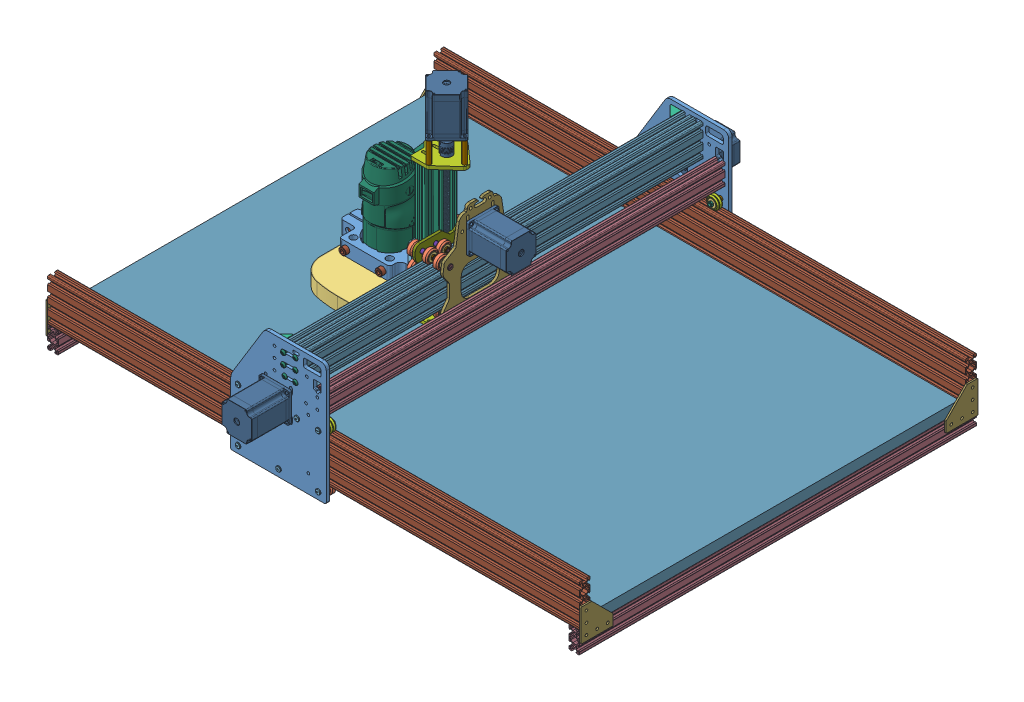
SolidWorks assembly MainFrame, configuration Default. Lengths in mm. (continued)
Components (placement in the parent): (continued)
- V-Slot_Nema23_Z_Build_Plate-1: V-Slot_Nema23_Z_Build_Plate [Default] at (-108.8467 132.9785 -347.7105) x (0 1 0) z (1 0 0) size (382.7 179.74 222.35) (hidden)
  - V-Slot NemaZ Build Plate-1: V-Slot NemaZ Build Plate [Default] at (-20.2121 124.8825 30.9396) size (88 127 2.54)
  - V-Slot Spacer Block-1: V-Slot Spacer Block [Default] at (-73.8059 59.9877 39.4796) x (1 0 0) z (0 0 1) size (86 20 12)
  - V-Slot Spacer Block-2: V-Slot Spacer Block [Default] at (-73.8059 -40.6523 39.4796) size (86 20 12)
  - 8mm Acme Nut Block-1: 8mm Acme Nut Block [Default] at (-83.4859 9.6677 39.4796) x (0 1 0) z (-1 0 0) size (34 12 20.51)
  - SolidWheelWithEccentric2-1: SolidWheelWithEccentric2 [Default] at (-136.732 -45.0423 82.73) x (-0.923728 -0.383049 0) z (0 0 -1) size (23.89 23.89 32.23)
    - SolidWheel-1: SolidWheel [Default] at (5.3595 -13.235 6.1636) size (23.89 23.89 11)
      - Delrin Solid V-Wheel-1: Delrin Solid V-Wheel [Default] at (-37.4558 4.6779 16.5868) size (23.89 23.89 10.23)
      - Precision Ball Bearing-1: Precision Ball Bearing [Default] at (-37.4558 4.6779 19.5868) x (0 0 -1) z (1 0 0) size (5 16 16)
      - Precision Ball Bearing-2: Precision Ball Bearing [Default] at (-37.4558 4.6779 13.5868) x (0 0 1) z (-1 0 0) size (5 16 16)
    - Steel Eccentric Spacer-1: Steel Eccentric Spacer [Default] at (-32.1017 -9.3471 37.2504) x (0 0 -1) z (0.00681 0.999977 0) size (7.27 9.09 7.9)
    - Low Profile Socket Head Screw-1: Low Profile Socket Head Screw [Default] at (-32.0963 -8.5571 45.0004) x (0 0 -1) z (1 0 0) size (32.23 9.5 9.5)
    - hex nut jam_am-1: hex nut jam_am [B18.2.4.5M - Hex jam nut,  M5 x 0.8 --D-N] at (-32.0963 -8.5571 17.2504) size (8 9.24 2.7)
    - 3mm Aluminum Spacer-1: 3mm Aluminum Spacer [Default] at (-32.0963 -8.5571 31.2504) x (0 0 -1) z (1 0 0) size (3 8 8)
  - SolidWheelWithEccentric2-2: SolidWheelWithEccentric2 [Default] at (-76.732 -45.0423 82.73) x (-0.923728 -0.383049 0) z (0 0 -1) size (23.89 23.89 32.23)
    - SolidWheel-1: SolidWheel [Default] at (5.3595 -13.235 6.1636) size (23.89 23.89 11)
      - Delrin Solid V-Wheel-1: Delrin Solid V-Wheel [Default] at (-37.4558 4.6779 16.5868) size (23.89 23.89 10.23)
      - Precision Ball Bearing-1: Precision Ball Bearing [Default] at (-37.4558 4.6779 19.5868) x (0 0 -1) z (1 0 0) size (5 16 16)
      - Precision Ball Bearing-2: Precision Ball Bearing [Default] at (-37.4558 4.6779 13.5868) x (0 0 1) z (-1 0 0) size (5 16 16)
    - Steel Eccentric Spacer-1: Steel Eccentric Spacer [Default] at (-32.1017 -9.3471 37.2504) x (0 0 -1) z (0.00681 0.999977 0) size (7.27 9.09 7.9)
    - Low Profile Socket Head Screw-1: Low Profile Socket Head Screw [Default] at (-32.0963 -8.5571 45.0004) x (0 0 -1) z (1 0 0) size (32.23 9.5 9.5)
    - hex nut jam_am-1: hex nut jam_am [B18.2.4.5M - Hex jam nut,  M5 x 0.8 --D-N] at (-32.0963 -8.5571 17.2504) size (8 9.24 2.7)
    - 3mm Aluminum Spacer-1: 3mm Aluminum Spacer [Default] at (-32.0963 -8.5571 31.2504) x (0 0 -1) z (1 0 0) size (3 8 8)
  - SolidWheelWithSpacer-1: SolidWheelWithSpacer [Default] at (-83.1141 65.4802 73.4636) x (0.923728 0.383049 0) z (0 0 -1) size (23.89 23.89 32.23)
    - SolidWheel-1: SolidWheel [Default] at (16.2383 -7.5303 -3.4528) size (23.89 23.89 11)
      - Delrin Solid V-Wheel-1: Delrin Solid V-Wheel [Default] at (-37.4558 4.6779 16.5868) size (23.89 23.89 10.23)
      - Precision Ball Bearing-1: Precision Ball Bearing [Default] at (-37.4558 4.6779 19.5868) x (0 0 -1) z (1 0 0) size (5 16 16)
      - Precision Ball Bearing-2: Precision Ball Bearing [Default] at (-37.4558 4.6779 13.5868) x (0 0 1) z (-1 0 0) size (5 16 16)
    - Low Profile Socket Head Screw-1: Low Profile Socket Head Screw [Default] at (-21.2174 -2.8524 35.734) x (0 0 -1) z (-0.923728 -0.383049 0) size (32.23 9.5 9.5)
    - .25 Inch Nylon Spacer-1: .25 Inch Nylon Spacer [Default] at (-21.2174 -2.8524 27.984) x (0 0 -1) z (1 0 0) size (6.35 7.94 7.94)
    - hex nut jam_am-1: hex nut jam_am [B18.2.4.5M - Hex jam nut,  M5 x 0.8 --D-N] at (-21.2174 -2.8524 7.634) size (8 9.24 2.7)
    - 3mm Aluminum Spacer-1: 3mm Aluminum Spacer [Default] at (-21.2174 -2.8524 21.634) x (0 0 -1) z (1 0 0) size (3 8 8)
  - SolidWheelWithSpacer-2: SolidWheelWithSpacer [Default] at (-64.4976 54.4952 73.4636) x (-0.923728 -0.383049 0) z (0 0 -1) size (23.89 23.89 32.23)
    - SolidWheel-1: SolidWheel [Default] at (16.2383 -7.5303 -3.4528) size (23.89 23.89 11)
      - Delrin Solid V-Wheel-1: Delrin Solid V-Wheel [Default] at (-37.4558 4.6779 16.5868) size (23.89 23.89 10.23)
      - Precision Ball Bearing-1: Precision Ball Bearing [Default] at (-37.4558 4.6779 19.5868) x (0 0 -1) z (1 0 0) size (5 16 16)
      - Precision Ball Bearing-2: Precision Ball Bearing [Default] at (-37.4558 4.6779 13.5868) x (0 0 1) z (-1 0 0) size (5 16 16)
    - Low Profile Socket Head Screw-1: Low Profile Socket Head Screw [Default] at (-21.2174 -2.8524 35.734) x (0 0 -1) z (-0.923728 -0.383049 0) size (32.23 9.5 9.5)
    - .25 Inch Nylon Spacer-1: .25 Inch Nylon Spacer [Default] at (-21.2174 -2.8524 27.984) x (0 0 -1) z (1 0 0) size (6.35 7.94 7.94)
    - hex nut jam_am-1: hex nut jam_am [B18.2.4.5M - Hex jam nut,  M5 x 0.8 --D-N] at (-21.2174 -2.8524 7.634) size (8 9.24 2.7)
    - 3mm Aluminum Spacer-1: 3mm Aluminum Spacer [Default] at (-21.2174 -2.8524 21.634) x (0 0 -1) z (1 0 0) size (3 8 8)
  - SolidWheelWithSpacer-3: SolidWheelWithSpacer [Default] at (-53.5632 53.0198 73.4636) x (0.980486 -0.196591 0) z (0 0 -1) size (23.89 23.89 32.23)
    - SolidWheel-1: SolidWheel [Default] at (16.2383 -7.5303 -3.4528) size (23.89 23.89 11)
      - Delrin Solid V-Wheel-1: Delrin Solid V-Wheel [Default] at (-37.4558 4.6779 16.5868) size (23.89 23.89 10.23)
      - Precision Ball Bearing-1: Precision Ball Bearing [Default] at (-37.4558 4.6779 19.5868) x (0 0 -1) z (1 0 0) size (5 16 16)
      - Precision Ball Bearing-2: Precision Ball Bearing [Default] at (-37.4558 4.6779 13.5868) x (0 0 1) z (-1 0 0) size (5 16 16)
    - Low Profile Socket Head Screw-1: Low Profile Socket Head Screw [Default] at (-21.2174 -2.8524 35.734) x (0 0 -1) z (-0.923728 -0.383049 0) size (32.23 9.5 9.5)
    - .25 Inch Nylon Spacer-1: .25 Inch Nylon Spacer [Default] at (-21.2174 -2.8524 27.984) x (0 0 -1) z (1 0 0) size (6.35 7.94 7.94)
    - hex nut jam_am-1: hex nut jam_am [B18.2.4.5M - Hex jam nut,  M5 x 0.8 --D-N] at (-21.2174 -2.8524 7.634) size (8 9.24 2.7)
    - 3mm Aluminum Spacer-1: 3mm Aluminum Spacer [Default] at (-21.2174 -2.8524 21.634) x (0 0 -1) z (1 0 0) size (3 8 8)
  - SolidWheelWithEccentric2-3: SolidWheelWithEccentric2 [Default] at (-106.732 -45.0423 82.73) x (-0.923728 -0.383049 0) z (0 0 -1) size (23.89 23.89 32.23)
    - SolidWheel-1: SolidWheel [Default] at (5.3595 -13.235 6.1636) size (23.89 23.89 11)
      - Delrin Solid V-Wheel-1: Delrin Solid V-Wheel [Default] at (-37.4558 4.6779 16.5868) size (23.89 23.89 10.23)
      - Precision Ball Bearing-1: Precision Ball Bearing [Default] at (-37.4558 4.6779 19.5868) x (0 0 -1) z (1 0 0) size (5 16 16)
      - Precision Ball Bearing-2: Precision Ball Bearing [Default] at (-37.4558 4.6779 13.5868) x (0 0 1) z (-1 0 0) size (5 16 16)
    - Steel Eccentric Spacer-1: Steel Eccentric Spacer [Default] at (-32.1017 -9.3471 37.2504) x (0 0 -1) z (0.00681 0.999977 0) size (7.27 9.09 7.9)
    - Low Profile Socket Head Screw-1: Low Profile Socket Head Screw [Default] at (-32.0963 -8.5571 45.0004) x (0 0 -1) z (1 0 0) size (32.23 9.5 9.5)
    - hex nut jam_am-1: hex nut jam_am [B18.2.4.5M - Hex jam nut,  M5 x 0.8 --D-N] at (-32.0963 -8.5571 17.2504) size (8 9.24 2.7)
    - 3mm Aluminum Spacer-1: 3mm Aluminum Spacer [Default] at (-32.0963 -8.5571 31.2504) x (0 0 -1) z (1 0 0) size (3 8 8)
  - 8mm TR8_8 Leadscrew-1: 8mm TR8_8 Leadscrew [1000mm - Default] at (-183.0043 9.6677 39.2196) x (0 0 1) z (-1 0 0) size (8.21 8.21 254)
  - V-Slot 20mm x 80mm x 300mm-1: V-Slot 20mm x 80mm x 300mm [Default] at (-184.3543 39.8452 60.1696) x (0 0 1) z (-1 0 0) size (20 80.02 250)
  - V-Slot Threaded Rod Plate-Nema23-1: V-Slot Threaded Rod Plate-Nema23 [Default] at (65.6457 -0.3323 60.1696) x (0 1 0) z (1 0 0) size (80 77.5 6.35)
  - V-Slot Threaded Rod Plate-Nema23-2: V-Slot Threaded Rod Plate-Nema23 [Default] at (-184.3543 19.6677 60.1696) x (0 -1 0) z (-1 0 0) size (80 77.5 6.35) (hidden)
  - stepper motor NEMA 23 57x76-1: stepper motor NEMA 23 57x76 [По умолчанию] at (186.9957 9.6677 39.2196) x (0 0.707107 -0.707107) z (0 0.707107 0.707107) size (56.67 96.5 56.58)
  - 40mm Aluminum Spacer-1: 40mm Aluminum Spacer [Default] at (111.9957 -23.9906 39.2196) x (-1 0 0) z (0 0.924225 0.381849) size (40 8 8)
  - 40mm Aluminum Spacer-2: 40mm Aluminum Spacer [Default] at (111.9957 9.6677 5.5613) x (-1 0 0) z (0 0.924225 0.381849) size (40 8 8)
  - 40mm Aluminum Spacer-3: 40mm Aluminum Spacer [Default] at (111.9957 43.326 39.2196) x (-1 0 0) z (0 0.924225 0.381849) size (40 8 8)
  - 40mm Aluminum Spacer-4: 40mm Aluminum Spacer [Default] at (111.9957 9.6677 72.8779) x (-1 0 0) z (0 0.924225 0.381849) size (40 8 8)
  - socket head cap screw_am-1: socket head cap screw_am [B18.3.1M - 5 x 0.8 x 25 Hex SHCS -- 25NHX] at (76.9957 -20.1748 60.1696) x (-1 0 0) z (0 -0.384278 0.923217) size (30 8.5 8.5)
  - socket head cap screw_am-2: socket head cap screw_am [B18.3.1M - 5 x 0.8 x 25 Hex SHCS -- 25NHX] at (76.9957 -0.1748 60.1696) x (-1 0 0) z (0 -0.700437 0.713714) size (30 8.5 8.5)
  - socket head cap screw_am-3: socket head cap screw_am [B18.3.1M - 5 x 0.8 x 25 Hex SHCS -- 25NHX] at (76.9957 19.8452 60.1696) x (-1 0 0) z (0 0.86302 0.50517) size (30 8.5 8.5)
  - socket head cap screw_am-4: socket head cap screw_am [B18.3.1M - 5 x 0.8 x 25 Hex SHCS -- 25NHX] at (76.9957 39.8452 60.1696) x (-1 0 0) z (0 0 1) size (30 8.5 8.5)
  - socket head cap screw_am-6: socket head cap screw_am [B18.3.1M - 5 x 0.8 x 25 Hex SHCS -- 25NHX] at (-195.7043 -20.1748 60.1696) x (1 0 0) z (0 0 1) size (30 8.5 8.5)
  - socket head cap screw_am-7: socket head cap screw_am [B18.3.1M - 5 x 0.8 x 25 Hex SHCS -- 25NHX] at (-195.7043 -0.1748 60.1696) x (1 0 0) z (0 0 1) size (30 8.5 8.5)
  - socket head cap screw_am-8: socket head cap screw_am [B18.3.1M - 5 x 0.8 x 25 Hex SHCS -- 25NHX] at (-195.7043 19.8452 60.1696) x (1 0 0) z (0 0 1) size (30 8.5 8.5)
  - socket head cap screw_am-9: socket head cap screw_am [B18.3.1M - 5 x 0.8 x 25 Hex SHCS -- 25NHX] at (-195.7043 39.8452 60.1696) x (1 0 0) z (0 0 1) size (30 8.5 8.5)
  - socket head cap screw_am-10: socket head cap screw_am [B18.3.1M - 4 x 0.7 x 55 Hex SHCS -- 20NHX] at (120.9957 -23.9906 39.2196) x (-1 0 0) z (0 0.924225 0.381849) size (59 7 7)
  - socket head cap screw_am-11: socket head cap screw_am [B18.3.1M - 4 x 0.7 x 55 Hex SHCS -- 20NHX] at (120.9957 9.6677 5.5613) x (-1 0 0) z (0 0 1) size (59 7 7)
  - socket head cap screw_am-12: socket head cap screw_am [B18.3.1M - 4 x 0.7 x 55 Hex SHCS -- 20NHX] at (120.9957 43.326 39.2196) x (-1 0 0) z (0 0 1) size (59 7 7)
  - socket head cap screw_am-13: socket head cap screw_am [B18.3.1M - 4 x 0.7 x 55 Hex SHCS -- 20NHX] at (120.9957 9.6677 72.8779) x (-1 0 0) z (0 0 1) size (59 7 7)
  - 5mm x 8mm Flexible Coupling-1: 5mm x 8mm Flexible Coupling [Default] at (76.9957 9.6677 39.2196) x (0 0 1) z (-1 0 0) size (20.7 20.83 25.02)
  - BoschRouter-1: BoschRouter [Default] at (-190.8659 -31.4315 -23.846) x (0 0 1) z (0 1 0) size (186 234.6 179.74) (hidden)
    - Main router body-1: Main router body [Default] at (-10.2226 84.5551 41.0992) size (99.4 181.94 153.51)
    - Part2^BoschRouter-1: Part2^BoschRouter [Default] at (-10.2226 69.8231 41.0992) x (-0.837169 0 -0.546944) z (-0.546944 0 0.837169) size (16.99 12.7 21.58) (virtual)
    - 0.25 in ENDMILL-1: 0.25 in ENDMILL [Default] at (-10.3095 59.0843 40.9903) x (-0.983799 0 0.179276) z (0.179276 0 0.983799) size (6.8 68.83 6.97)
    - pan cross head_ai-1: pan cross head_ai [CR-PHMS 0.138-32x0.375x0.375-N] at (-1.965 82.0913 10.6382) x (0 1 0) z (0 0 1) size (11.95 6.86 6.86)
    - pan cross head_ai-2: pan cross head_ai [CR-PHMS 0.138-32x0.375x0.375-N] at (-41.774 82.0913 41.8547) x (0 1 0) z (0 0 1) size (11.95 6.86 6.86)
    - pan cross head_ai-3: pan cross head_ai [CR-PHMS 0.138-32x0.375x0.375-N] at (9.6999 82.0913 65.5768) x (0 1 0) z (0 0 1) size (11.95 6.86 6.86)
    - BoschRouterMount-1: BoschRouterMount [Default] at (-10.2226 84.5551 41.0992) x (-1 0 0) z (0 -1 0) size (140 100 25)
    - socket head cap screw_am-1: socket head cap screw_am [B18.3.1M - 8 x 1.25 x 30 Hex SHCS -- 30NHX] at (-70.2144 97.0551 17.7105) x (0 0 1) z (0.923728 0.383049 0) size (38 13 13)
    - BoschRouter-ShoeRods-1: BoschRouter-ShoeRods [Default] at (-10.2226 109.5551 41.0992) x (1 0 0) z (0 1 0) size (80.73 12.7 110)
    - BoschRouter-ShowPlate-1: BoschRouter-ShowPlate [Default] at (-10.2226 32.6551 41.0992) x (-1 0 0) z (0 -1 0) size (162 139.64 25.4)
    - socket head cap screw_am-2: socket head cap screw_am [B18.3.1M - 8 x 1.25 x 12 Hex SHCS -- 12NHX] at (26.3004 97.0551 98.7105) x (0 0 -1) z (1 0 0) size (20 13 13)
    - socket head cap screw_am-3: socket head cap screw_am [B18.3.1M - 8 x 1.25 x 12 Hex SHCS -- 12NHX] at (-41.7291 97.0551 98.7105) x (0 0 -1) z (1 0 0) size (20 13 13)
    - socket head cap screw_am-4: socket head cap screw_am [B18.3.1M - 8 x 1.25 x 12 Hex SHCS -- 12NHX] at (26.3004 97.0551 -17.2895) x (0 0 1) z (-1 0 0) size (20 13 13)
    - socket head cap screw_am-5: socket head cap screw_am [B18.3.1M - 8 x 1.25 x 12 Hex SHCS -- 12NHX] at (-41.7291 97.0551 -17.2895) x (0 0 1) z (-1 0 0) size (20 13 13)
    - BoschRouter-ShoeVacumPort-1: BoschRouter-ShoeVacumPort [Default] at (-10.2226 32.6551 41.0992) x (1 0 0) z (0 1 0) size (45 45 44.53)
    - RouterMountingPlate-2: RouterMountingPlate [Default] at (-25.2226 46.2551 41.0992) x (1 0 0) z (0 1 0) size (6.35 60 101.6)
    - socket head cap screw_am-6: socket head cap screw_am [B18.3.1M - 5 x 0.8 x 12 Hex SHCS -- 12NHX] at (49.7856 137.8551 61.0992) size (17 8.5 8.5)
    - socket head cap screw_am-7: socket head cap screw_am [B18.3.1M - 5 x 0.8 x 12 Hex SHCS -- 12NHX] at (49.7856 137.8551 41.0992) size (17 8.5 8.5)
    - socket head cap screw_am-8: socket head cap screw_am [B18.3.1M - 5 x 0.8 x 12 Hex SHCS -- 12NHX] at (49.7856 137.8551 21.0992) size (17 8.5 8.5)
    - socket head cap screw_am-9: socket head cap screw_am [B18.3.1M - 5 x 0.8 x 12 Hex SHCS -- 12NHX] at (49.7856 56.2551 21.0992) x (1 0 0) z (0 0 -1) size (17 8.5 8.5)
    - socket head cap screw_am-10: socket head cap screw_am [B18.3.1M - 5 x 0.8 x 12 Hex SHCS -- 12NHX] at (49.7856 56.2551 61.0992) size (17 8.5 8.5)
    - socket head cap screw_am-11: socket head cap screw_am [B18.3.1M - 5 x 0.8 x 12 Hex SHCS -- 12NHX] at (49.7856 56.2551 41.0992) size (17 8.5 8.5)
  - V-Slot_Bottom_Threaded_Rod_Plate-Nema23-1: V-Slot_Bottom_Threaded_Rod_Plate-Nema23 [Default] at (-184.3543 19.6677 60.1696) x (0 -1 0) z (-1 0 0) size (80 45 6.35)
  - R4-ZZ Ball Bearing-1: R4-ZZ Ball Bearing [Default] at (-184.8651 9.6677 39.2196) x (1 0 0) z (0 0 1) size (4.98 10 10)
  - R4-ZZ Ball Bearing-2: R4-ZZ Ball Bearing [Default] at (65.1349 9.6677 39.2196) x (1 0 0) z (0 0.062023 0.998075) size (4.98 10 10)
- 5 Hole 90 Degree Joining Plate-1: 5 Hole 90 Degree Joining Plate [Default] at (-476.3518 -111.2884 -724.722) x (0 0 1) z (-0.999999 -0.001454 0) size (60 60 3)
- 5 Hole 90 Degree Joining Plate-2: 5 Hole 90 Degree Joining Plate [Default] at (-473.3518 -111.284 21.278) x (0 0 -1) z (0.999999 0.001454 0) size (60 60 3)
- 5 Hole 90 Degree Joining Plate-3: 5 Hole 90 Degree Joining Plate [Default] at (526.6471 -109.8153 -724.7365) x (0.000002 -0.001454 0.999999) z (-0.999999 -0.001454 0) size (60 60 3)
- 5 Hole 90 Degree Joining Plate-4: 5 Hole 90 Degree Joining Plate [Default] at (529.6471 -109.8255 21.278) x (0 0 -1) z (0.999999 0.001454 0) size (60 60 3)
- V-Slot 20mm x 40mm x BedCrossBrace-1: V-Slot 20mm x 40mm x BedCrossBrace [Default] at (516.632 -99.4444 21.278) x (0.999999 0.001454 0) z (0 0 1) size (20 40 746)
- V-Slot 20mm x 40mm x BedCrossBrace-4: V-Slot 20mm x 40mm x BedCrossBrace [Default] at (-463.367 -100.8695 21.278) x (0.999999 0.001454 0) z (0 0 1) size (20 40 746)
- HoldDownBoard-1: HoldDownBoard [Default] at (196.6178 -89.9123 21.278) x (0.999999 0.001454 0) z (-0.001454 0.999999 0) size (1000 680.6 19.05)
- BoschRouter-2: BoschRouter [Default] at (-136.4727 -50.9445 -335.8021) x (1 0 0) z (0 -0.000396 1) size (186 234.6 179.74)
  - Main router body-1: Main router body [Default] at (-10.2226 84.5551 41.0992) size (99.4 181.94 153.51)
  - Part2^BoschRouter-1: Part2^BoschRouter [Default] at (-10.2226 69.8231 41.0992) x (-0.837169 0 -0.546944) z (-0.546944 0 0.837169) size (16.99 12.7 21.58) (virtual)
  - 0.25 in ENDMILL-1: 0.25 in ENDMILL [Default] at (-10.3095 59.0843 40.9903) x (-0.983799 0 0.179276) z (0.179276 0 0.983799) size (6.8 68.83 6.97)
  - pan cross head_ai-1: pan cross head_ai [CR-PHMS 0.138-32x0.375x0.375-N] at (-1.965 82.0913 10.6382) x (0 1 0) z (0 0 1) size (11.95 6.86 6.86)
  - pan cross head_ai-2: pan cross head_ai [CR-PHMS 0.138-32x0.375x0.375-N] at (-41.774 82.0913 41.8547) x (0 1 0) z (0 0 1) size (11.95 6.86 6.86)
  - pan cross head_ai-3: pan cross head_ai [CR-PHMS 0.138-32x0.375x0.375-N] at (9.6999 82.0913 65.5768) x (0 1 0) z (0 0 1) size (11.95 6.86 6.86)
  - BoschRouterMount-1: BoschRouterMount [Default] at (-10.2226 84.5551 41.0992) x (-1 0 0) z (0 -1 0) size (140 100 25)
  - socket head cap screw_am-1: socket head cap screw_am [B18.3.1M - 8 x 1.25 x 30 Hex SHCS -- 30NHX] at (-70.2144 97.0551 17.7105) x (0 0 1) z (0.923728 0.383049 0) size (38 13 13)
  - BoschRouter-ShoeRods-1: BoschRouter-ShoeRods [Default] at (-10.2226 109.5551 41.0992) x (1 0 0) z (0 1 0) size (80.73 12.7 110)
  - BoschRouter-ShowPlate-1: BoschRouter-ShowPlate [Default] at (-10.2226 32.6551 41.0992) x (-1 0 0) z (0 -1 0) size (162 139.64 25.4)
  - socket head cap screw_am-2: socket head cap screw_am [B18.3.1M - 8 x 1.25 x 12 Hex SHCS -- 12NHX] at (26.3004 97.0551 98.7105) x (0 0 -1) z (1 0 0) size (20 13 13)
  - socket head cap screw_am-3: socket head cap screw_am [B18.3.1M - 8 x 1.25 x 12 Hex SHCS -- 12NHX] at (-41.7291 97.0551 98.7105) x (0 0 -1) z (1 0 0) size (20 13 13)
  - socket head cap screw_am-4: socket head cap screw_am [B18.3.1M - 8 x 1.25 x 12 Hex SHCS -- 12NHX] at (26.3004 97.0551 -17.2895) x (0 0 1) z (-1 0 0) size (20 13 13)
  - socket head cap screw_am-5: socket head cap screw_am [B18.3.1M - 8 x 1.25 x 12 Hex SHCS -- 12NHX] at (-41.7291 97.0551 -17.2895) x (0 0 1) z (-1 0 0) size (20 13 13)
  - BoschRouter-ShoeVacumPort-1: BoschRouter-ShoeVacumPort [Default] at (-10.2226 32.6551 41.0992) x (1 0 0) z (0 1 0) size (45 45 44.53)
  - RouterMountingPlate-2: RouterMountingPlate [Default] at (-25.2226 46.2551 41.0992) x (1 0 0) z (0 1 0) size (6.35 60 101.6)
  - socket head cap screw_am-6: socket head cap screw_am [B18.3.1M - 5 x 0.8 x 12 Hex SHCS -- 12NHX] at (49.7856 137.8551 61.0992) size (17 8.5 8.5)
  - socket head cap screw_am-7: socket head cap screw_am [B18.3.1M - 5 x 0.8 x 12 Hex SHCS -- 12NHX] at (49.7856 137.8551 41.0992) size (17 8.5 8.5)
  - socket head cap screw_am-8: socket head cap screw_am [B18.3.1M - 5 x 0.8 x 12 Hex SHCS -- 12NHX] at (49.7856 137.8551 21.0992) size (17 8.5 8.5)
  - socket head cap screw_am-9: socket head cap screw_am [B18.3.1M - 5 x 0.8 x 12 Hex SHCS -- 12NHX] at (49.7856 56.2551 21.0992) x (1 0 0) z (0 0 -1) size (17 8.5 8.5)
  - socket head cap screw_am-10: socket head cap screw_am [B18.3.1M - 5 x 0.8 x 12 Hex SHCS -- 12NHX] at (49.7856 56.2551 61.0992) size (17 8.5 8.5)
  - socket head cap screw_am-11: socket head cap screw_am [B18.3.1M - 5 x 0.8 x 12 Hex SHCS -- 12NHX] at (49.7856 56.2551 41.0992) size (17 8.5 8.5)
- V-Slot 20mm x 40mm x BedCrossBrace-5: V-Slot 20mm x 40mm x BedCrossBrace [Default] at (42.0876 32.3489 19.278) x (-0.999999 -0.001454 0) z (0 0 1) size (20 40 746)
- Cast - 90 Degree Corner Bracket-1: Cast - 90 Degree Corner Bracket [Default] at (-29.1646 95.8532 23.278) x (0 0 -1) z (0 1 0) size (20.75 20.75 20)
- Cast - 90 Degree Corner Bracket-2: Cast - 90 Degree Corner Bracket [Default] at (-29.1646 55.8235 23.278) x (0 0 -1) z (0 1 0) size (20.75 20.75 20)
- Cast - 90 Degree Corner Bracket-3: Cast - 90 Degree Corner Bracket [Default] at (-29.1646 75.8532 23.278) x (0 0 -1) z (0 1 0) size (20.75 20.75 20)
- Cast - 90 Degree Corner Bracket-4: Cast - 90 Degree Corner Bracket [Default] at (-29.1646 75.8532 -726.722) x (-1 0 0) z (0 1 0) size (20.75 20.75 20)
- Cast - 90 Degree Corner Bracket-5: Cast - 90 Degree Corner Bracket [Default] at (-29.1646 55.8235 -726.722) x (-1 0 0) z (0 1 0) size (20.75 20.75 20)
- Cast - 90 Degree Corner Bracket-6: Cast - 90 Degree Corner Bracket [Default] at (-29.1646 95.8532 -726.722) x (-1 0 0) z (0 1 0) size (20.75 20.75 20)
Mates (geometry in assembly coordinates):
- Tangent11: tangent aligned: cylinder of LeftSideGantry-1/V-Slot Delrin Dual Wheel Assembly-1/Delrin Dual V-Wheel-1 through (-106.5524 -0.6055 16.543) axis (0 0 1) radius 11.945; plane of vslot_20_x_80-1 through (-473.4946 -13.0842 8.438) normal (0.001454 -0.999999 0)
- Tangent12: tangent aligned: cylinder of LeftSideGantry-1/V-Slot Delrin Dual Wheel Assembly-3/Delrin Dual V-Wheel-1 through (44.0424 -0.3866 16.543) axis (0 0 1) radius 11.945; plane of vslot_20_x_80-1 through (-473.4946 -13.0842 8.438) normal (0.001454 -0.999999 0)
- Distance1: distance = 2 mm anti-aligned: plane of vslot_20_x_80-1 through (-473.3887 -85.9241 21.278) normal (0 0 1); plane of LeftSideGantry-1/Gantry-SidePlate-1 through (-117.8896 -110.2681 23.278) normal (0 0 -1)
- Coincident4: coincident aligned: plane of LeftSideGantry-1/Gantry-SidePlate-1 through (-50.0596 113.859 29.628) normal (0 1 0); plane of RightSideGantry-1/Gantry-SidePlate-1 through (-50.0596 113.859 -726.722) normal (0 1 0)
- Coincident5: coincident aligned: plane of LeftSideGantry-1/Gantry-SidePlate-1 through (-121.2524 -110.2681 29.628) normal (-1 0 0); plane of RightSideGantry-1/Gantry-SidePlate-1 through (-121.2524 -110.2681 -726.722) normal (-1 0 0)
- Coincident6: coincident aligned: plane of vslot_20_x_80-1 through (-473.4973 -11.2842 3.278) normal (-0.001454 0.999999 0); plane of vslot_20_x_80-2 through (-473.4973 -11.2842 -710.082) normal (-0.001454 0.999999 0)
- Distance2: distance = 2 mm anti-aligned: plane of vslot_20_x_80-2 through (-473.4604 -36.6441 -724.722) normal (0 0 -1); plane of RightSideGantry-1/Gantry-SidePlate-1 through (-117.8896 -110.2681 -726.722) normal (0 0 1)
- Coincident8: coincident aligned: plane of vslot_20_x_80-1 through (-473.4944 -13.2842 3.278) normal (-0.999999 -0.001454 0); plane of vslot_20_x_80-2 through (-473.4944 -13.2842 -722.722) normal (-0.999999 -0.001454 0)
- Distance3: distance = 750 mm anti-aligned: plane of LeftSideGantry-1/Gantry-SidePlate-1 through (-117.8896 -110.2681 23.278) normal (0 0 -1); plane of RightSideGantry-1/Gantry-SidePlate-1 through (-117.8896 -110.2681 -726.722) normal (0 0 1)
- Coincident9: coincident anti-aligned: plane of vslot 20 x 60-1/vslot_20_x_60-1 through (-9.1646 61.0231 86.5236) normal (-1 0 0); plane of vslot 20 x 60-2/vslot_20_x_60-1 through (-9.1646 61.0231 -789.9675) normal (1 0 0)
- Concentric1: concentric anti-aligned: cylinder of LeftSideGantry-1/Gantry-SidePlate-1 through (-19.1646 96.383 29.628) axis (0 0 -1) radius 2.5; cylinder of vslot 20 x 60-2/socket button head cap screw_am-3 through (-19.1646 96.3831 34.778) axis (0 0 1) radius 2.5
- Concentric2: concentric anti-aligned: cylinder of LeftSideGantry-1/Gantry-SidePlate-1 through (-19.1646 56.3831 29.628) axis (0 0 -1) radius 2.5; cylinder of vslot 20 x 60-2/socket button head cap screw_am-1 through (-19.1646 56.3831 32.028) axis (0 0 1) radius 2.5
- Coincident11: coincident anti-aligned: plane of LeftSideGantry-1/Gantry-SidePlate-1 through (-117.8896 -110.2681 23.278) normal (0 0 -1); plane of vslot 20 x 60-2/vslot_20_x_60-1 through (-27.3646 48.1831 23.278) normal (0 0 1)
- Coincident12: coincident anti-aligned: plane of RightSideGantry-1/Gantry-SidePlate-1 through (-117.8896 -110.2681 -726.722) normal (0 0 1); plane of vslot 20 x 60-1/vslot_20_x_60-1 through (9.0354 48.1831 -726.722) normal (0 0 -1)
- Coincident13: coincident aligned: plane of vslot 20 x 60-1/vslot_20_x_60-1 through (5.4754 106.3831 86.5236) normal (0 1 0); plane of vslot 20 x 60-2/vslot_20_x_60-1 through (-10.9646 106.3831 -789.9675) normal (0 1 0)
- Tangent14: tangent aligned: cylinder of CrossSlideAssembly-1/SolidWheel-9/Delrin Solid V-Wheel-1 through (-4.1796 116.5281 -357.1491) axis (-1 0 0) radius 11.945; plane of vslot 20 x 60-1/vslot_20_x_60-1 through (-2.0046 104.5831 86.5236) normal (0 -1 0)
- Tangent15: tangent anti-aligned: cone of CrossSlideAssembly-1/SolidWheel-9/Delrin Solid V-Wheel-1 through (-2.0046 116.5281 -357.1491) axis (-1 0 0); plane of vslot 20 x 60-1/vslot_20_x_60-1 through (-3.8046 106.3831 86.5236) normal (0.707107 0.707107 0)
- Concentric3: concentric aligned: circle of CrossSlideAssembly-1/SolidWheel-8/Delrin Solid V-Wheel-1; circle of FrontGantryPlateZaxis-1/SolidWheelWithSpacer-5/SolidWheel-1/Delrin Solid V-Wheel-1
- Tangent18: tangent aligned: cylinder of CrossSlideAssembly-1/SolidWheel-9/Delrin Solid V-Wheel-1 through (-4.1796 116.5281 -357.1491) axis (-1 0 0) radius 11.945; plane of vslot 20 x 60-1/vslot_20_x_60-1 through (6.3347 104.5831 86.5236) normal (0 -1 0)
- Tangent19: tangent aligned: cylinder of CrossSlideAssembly-1/SolidWheel-8/Delrin Solid V-Wheel-1 through (-4.1796 116.5281 -243.3829) axis (-1 0 0) radius 11.945; plane of vslot 20 x 60-1/vslot_20_x_60-1 through (-2.0046 104.5831 86.5236) normal (0 -1 0)
- Tangent20: tangent aligned: plane of vslot 20 x 60-2/vslot_20_x_60-1 through (-24.6639 104.5831 -789.9675) normal (0 -1 0); cylinder of FrontGantryPlateZaxis-1/SolidWheelWithSpacer-4/SolidWheel-1/Delrin Solid V-Wheel-1 through (-24.1796 116.5281 -357.2291) axis (-1 0 0) radius 11.945
- Tangent21: tangent anti-aligned: plane of vslot 20 x 60-2/vslot_20_x_60-1 through (-22.0046 104.5831 -789.9675) normal (0.707107 0.707107 0); cone of FrontGantryPlateZaxis-1/SolidWheelWithSpacer-4/SolidWheel-1/Delrin Solid V-Wheel-1 through (-22.0046 116.5281 -357.2291) axis (-1 0 0)
- Parallel1: parallel anti-aligned: plane of FrontGantryPlateZaxis-1/Gantry-Mount-Part2-1 through (-38.6771 130.1787 -360.7197) normal (0 1 0); plane of V-Slot_Nema23_Z_Build_Plate-1/V-Slot_Bottom_Threaded_Rod_Plate-Nema23-1 through (-78.6771 -57.7259 -373.0428) normal (0 -1 0)
- Coincident15: coincident anti-aligned: plane of FrontGantryPlateZaxis-1/Gantry-Mount-Part2-1 through (-38.6771 26.8255 -233.6488) normal (-1 0 0); plane of V-Slot_Nema23_Z_Build_Plate-1/V-Slot 20mm x 80mm x 300mm-1 through (-38.6771 198.6241 -342.9753) normal (1 0 0)
- Concentric4: concentric anti-aligned: cylinder of vslot_20_x_80-2 through (-473.4246 -61.2841 -714.722) axis (0.999999 0.001454 0) radius 2.1; cylinder of 5 Hole 90 Degree Joining Plate-1 through (-473.4246 -61.2841 -714.722) axis (-0.999999 -0.001454 0) radius 2.5
- Concentric5: concentric anti-aligned: cylinder of vslot_20_x_80-2 through (-473.3955 -81.2841 -714.722) axis (0.999999 0.001454 0) radius 2.1; cylinder of 5 Hole 90 Degree Joining Plate-1 through (-473.3955 -81.2841 -714.722) axis (-0.999999 -0.001454 0) radius 2.5
- Coincident16: coincident anti-aligned: plane of vslot_20_x_80-2 through (-473.4944 -13.2842 -722.722) normal (-0.999999 -0.001454 0); plane of 5 Hole 90 Degree Joining Plate-1 through (-473.38 -91.9054 -666.222) normal (0.999999 0.001454 0)
- Concentric6: concentric aligned: cylinder of vslot_20_x_80-1 through (-473.4246 -61.2841 11.278) axis (0.999999 0.001454 0) radius 2.1; cylinder of 5 Hole 90 Degree Joining Plate-2 through (-476.4246 -61.2885 11.278) axis (0.999999 0.001454 0) radius 2.5
- Concentric7: concentric aligned: cylinder of vslot_20_x_80-1 through (-473.3955 -81.2841 11.278) axis (0.999999 0.001454 0) radius 2.1; cylinder of 5 Hole 90 Degree Joining Plate-2 through (-476.3955 -81.2884 11.278) axis (0.999999 0.001454 0) radius 2.5
- Coincident17: coincident anti-aligned: plane of vslot_20_x_80-1 through (-473.4944 -13.2842 3.278) normal (-0.999999 -0.001454 0); plane of 5 Hole 90 Degree Joining Plate-2 through (-473.38 -91.9054 -37.222) normal (0.999999 0.001454 0)
- Concentric9: concentric aligned: cylinder of 5 Hole 90 Degree Joining Plate-1 through (-473.3664 -101.2841 -714.722) axis (-0.999999 -0.001454 0) radius 2.5; cylinder of 5 Hole 90 Degree Joining Plate-3 through (529.6326 -99.8255 -714.722) axis (-0.999999 -0.001454 0) radius 2.5
- Coincident18: coincident anti-aligned: plane of vslot_20_x_80-2 through (526.5046 -11.83 -722.722) normal (0.999999 0.001454 0); plane of 5 Hole 90 Degree Joining Plate-3 through (526.619 -90.5218 -666.2084) normal (-0.999999 -0.001454 0)
- Coincident21: coincident anti-aligned: plane of vslot_20_x_80-1 through (526.5046 -11.83 3.278) normal (0.999999 0.001454 0); plane of 5 Hole 90 Degree Joining Plate-4 through (526.6189 -90.4512 -37.222) normal (-0.999999 -0.001454 0)
- Concentric10: concentric aligned: cylinder of vslot_20_x_80-1 through (-473.4246 -61.2841 11.278) axis (0.999999 0.001454 0) radius 2.1; cylinder of 5 Hole 90 Degree Joining Plate-4 through (526.5744 -59.8299 11.278) axis (0.999999 0.001454 0) radius 2.5
- Concentric11: concentric aligned: cylinder of 5 Hole 90 Degree Joining Plate-2 through (-476.3955 -81.2884 11.278) axis (0.999999 0.001454 0) radius 2.5; cylinder of 5 Hole 90 Degree Joining Plate-4 through (526.6035 -79.8299 11.278) axis (0.999999 0.001454 0) radius 2.5
- Coincident22: coincident aligned: plane of 5 Hole 90 Degree Joining Plate-3 through (529.619 -90.5174 -666.2084) normal (0.999999 0.001454 0); plane of 5 Hole 90 Degree Joining Plate-4 through (529.6189 -90.4469 -37.222) normal (0.999999 0.001454 0)
- Coincident23: coincident aligned: plane of vslot_20_x_80-1 through (526.5046 -11.83 3.278) normal (0.999999 0.001454 0); plane of vslot_20_x_80-2 through (526.5046 -11.83 -722.722) normal (0.999999 0.001454 0)
- Coincident24: coincident aligned: plane of vslot_20_x_80-1 through (-473.4973 -11.2842 15.918) normal (-0.001454 0.999999 0); plane of vslot_20_x_80-2 through (-473.4973 -11.2842 -722.722) normal (-0.001454 0.999999 0)
- Coincident25: coincident aligned: plane of vslot_20_x_80-1 through (-473.4178 -65.9241 21.278) normal (0 0 1); plane of V-Slot 20mm x 40mm x BedCrossBrace-1 through (511.7114 -90.2441 21.278) normal (0 0 1)
- Coincident26: coincident anti-aligned: plane of 5 Hole 90 Degree Joining Plate-4 through (526.6189 -90.4512 -37.222) normal (-0.999999 -0.001454 0); plane of V-Slot 20mm x 40mm x BedCrossBrace-1 through (526.6391 -104.3413 -769.4389) normal (0.999999 0.001454 0)
- Tangent22: tangent aligned: cylinder of 5 Hole 90 Degree Joining Plate-4 through (526.6326 -99.8299 11.278) axis (0.999999 0.001454 0) radius 2.5; cylinder of V-Slot 20mm x 40mm x BedCrossBrace-1 through (516.632 -99.4444 -769.4389) axis (0 0 1) radius 2.1
- Coincident29: coincident aligned: plane of vslot_20_x_80-1 through (-473.4469 -45.9241 21.278) normal (0 0 1); plane of V-Slot 20mm x 40mm x BedCrossBrace-4 through (-468.2876 -91.6692 21.278) normal (0 0 1)
- Coincident30: coincident aligned: plane of V-Slot 20mm x 40mm x BedCrossBrace-1 through (511.7102 -89.4541 -769.4389) normal (-0.001454 0.999999 0); plane of V-Slot 20mm x 40mm x BedCrossBrace-4 through (-468.2887 -90.8792 -769.4389) normal (-0.001454 0.999999 0)
- Coincident31: coincident anti-aligned: plane of 5 Hole 90 Degree Joining Plate-2 through (-473.38 -91.9054 -37.222) normal (0.999999 0.001454 0); plane of V-Slot 20mm x 40mm x BedCrossBrace-4 through (-473.3598 -105.7954 -769.4389) normal (-0.999999 -0.001454 0)
- Coincident40: coincident anti-aligned: plane of FrontGantryPlateZaxis-1/V-Slot 20mm x 60mm x 300mm-1 through (-75.3371 -14.6973 -315.8772) normal (-1 0 0); plane of BoschRouter-2/RouterMountingPlate-2 through (-75.3371 96.9062 -324.6443) normal (1 0 0)
- Coincident41: coincident aligned: plane of FrontGantryPlateZaxis-1/V-Slot 20mm x 60mm x 300mm-1 through (-65.2371 -14.6938 -324.6885) normal (0 0.000396 -1); plane of BoschRouter-2/RouterMountingPlate-2 through (-81.6871 96.9062 -324.6443) normal (0 0.000396 -1)
- Distance4: distance = 10 mm anti-aligned: plane of BoschRouter-2/RouterMountingPlate-2 through (-161.6953 -4.7057 -294.6846) normal (0 -1 -0.000396); plane of FrontGantryPlateZaxis-1/V-Slot Threaded Rod Plate-Nema23-V2-2 through (-10.3371 -14.7024 -302.8687) normal (0 1 0.000396)
- Coincident44: coincident anti-aligned: plane of RightSideGantry-1/Gantry-SidePlate-1 through (-117.8896 -110.2681 -726.722) normal (0 0 1); plane of V-Slot 20mm x 40mm x BedCrossBrace-5 through (1032.209 -50.4514 -726.722) normal (0 0 -1)
- Concentric13: concentric anti-aligned: cylinder of RightSideGantry-1/Gantry-SidePlate-1 through (42.0876 32.3489 -726.722) axis (0 0 -1) radius 2.5006; cylinder of V-Slot 20mm x 40mm x BedCrossBrace-5 through (42.0876 32.3489 -771.4389) axis (0 0 1) radius 2.1
- Parallel4: parallel anti-aligned: plane of vslot_20_x_80-2 through (-473.4973 -11.2842 -710.082) normal (-0.001454 0.999999 0); plane of V-Slot 20mm x 40mm x BedCrossBrace-5 through (37.1949 22.3443 -771.4389) normal (0.001454 -0.999999 0)
- Coincident47: coincident anti-aligned: plane of vslot 20 x 60-2/vslot_20_x_60-1 through (-29.1646 91.7431 -789.9675) normal (-1 0 0); plane of Cast - 90 Degree Corner Bracket-4 through (-29.1646 85.8532 -726.722) normal (1 0 0)
- Coincident48: coincident anti-aligned: plane of RightSideGantry-1/Gantry-SidePlate-1 through (-117.8896 -110.2681 -726.722) normal (0 0 1); plane of Cast - 90 Degree Corner Bracket-4 through (-48.9146 85.8532 -726.722) normal (0 0 -1)
- Coincident49: coincident anti-aligned: plane of vslot 20 x 60-2/vslot_20_x_60-1 through (-29.1646 71.7431 -789.9675) normal (-1 0 0); plane of Cast - 90 Degree Corner Bracket-5 through (-29.1646 65.8235 -726.722) normal (1 0 0)
- Coincident50: coincident anti-aligned: plane of RightSideGantry-1/Gantry-SidePlate-1 through (-117.8896 -110.2681 -726.722) normal (0 0 1); plane of Cast - 90 Degree Corner Bracket-5 through (-48.9146 65.8235 -726.722) normal (0 0 -1)
- Coincident51: coincident anti-aligned: plane of vslot 20 x 60-2/vslot_20_x_60-1 through (-29.1646 71.7431 -789.9675) normal (-1 0 0); plane of Cast - 90 Degree Corner Bracket-6 through (-29.1646 105.8532 -726.722) normal (1 0 0)
- Coincident52: coincident anti-aligned: plane of RightSideGantry-1/Gantry-SidePlate-1 through (-117.8896 -110.2681 -726.722) normal (0 0 1); plane of Cast - 90 Degree Corner Bracket-6 through (-48.9146 105.8532 -726.722) normal (0 0 -1)
- Tangent23: tangent anti-aligned: cylinder of RightSideGantry-1/Gantry-SidePlate-1 through (-38.5217 56.3241 -726.722) axis (0 0 -1) radius 2.5006; plane of Cast - 90 Degree Corner Bracket-5 through (-38.4146 53.8235 -726.722) normal (0 1 0)
- Tangent24: tangent anti-aligned: cylinder of RightSideGantry-1/Gantry-SidePlate-1 through (-38.5217 96.3538 -726.722) axis (0 0 -1) radius 2.5006; plane of Cast - 90 Degree Corner Bracket-6 through (-38.4146 93.8532 -726.722) normal (0 1 0)
- Tangent25: tangent anti-aligned: cylinder of RightSideGantry-1/Gantry-SidePlate-1 through (-38.5217 76.3538 -726.722) axis (0 0 -1) radius 2.5006; plane of Cast - 90 Degree Corner Bracket-4 through (-38.4146 73.8532 -726.722) normal (0 1 0)
- Coincident53: coincident anti-aligned: plane of LeftSideGantry-1/Gantry-SidePlate-1 through (-117.8896 -110.2681 23.278) normal (0 0 -1); plane of Cast - 90 Degree Corner Bracket-3 through (-29.1646 85.8532 23.278) normal (0 0 1)
- Coincident54: coincident anti-aligned: plane of LeftSideGantry-1/Gantry-SidePlate-1 through (-117.8896 -110.2681 23.278) normal (0 0 -1); plane of Cast - 90 Degree Corner Bracket-2 through (-29.1646 65.8235 23.278) normal (0 0 1)
- Coincident55: coincident anti-aligned: plane of LeftSideGantry-1/Gantry-SidePlate-1 through (-117.8896 -110.2681 23.278) normal (0 0 -1); plane of Cast - 90 Degree Corner Bracket-1 through (-29.1646 105.8532 23.278) normal (0 0 1)
- Coincident56: coincident anti-aligned: plane of vslot 20 x 60-2/vslot_20_x_60-1 through (-29.1646 91.7431 -789.9675) normal (-1 0 0); plane of Cast - 90 Degree Corner Bracket-3 through (-29.1646 85.8532 3.528) normal (1 0 0)
- Tangent26: tangent anti-aligned: cylinder of LeftSideGantry-1/Gantry-SidePlate-1 through (-38.5217 76.3538 29.628) axis (0 0 -1) radius 2.5006; plane of Cast - 90 Degree Corner Bracket-3 through (-38.4146 73.8532 23.278) normal (0 1 0)
- Coincident57: coincident anti-aligned: plane of vslot 20 x 60-2/vslot_20_x_60-1 through (-29.1646 71.7431 -789.9675) normal (-1 0 0); plane of Cast - 90 Degree Corner Bracket-2 through (-29.1646 65.8235 3.528) normal (1 0 0)
- Tangent27: tangent anti-aligned: cylinder of LeftSideGantry-1/Gantry-SidePlate-1 through (-38.5217 56.3241 29.628) axis (0 0 -1) radius 2.5006; plane of Cast - 90 Degree Corner Bracket-2 through (-38.4146 53.8235 23.278) normal (0 1 0)
- Coincident58: coincident anti-aligned: plane of vslot 20 x 60-2/vslot_20_x_60-1 through (-29.1646 91.7431 -789.9675) normal (-1 0 0); plane of Cast - 90 Degree Corner Bracket-1 through (-29.1646 105.8532 3.528) normal (1 0 0)
- Tangent28: tangent anti-aligned: cylinder of LeftSideGantry-1/Gantry-SidePlate-1 through (-38.5217 96.3538 29.628) axis (0 0 -1) radius 2.5006; plane of Cast - 90 Degree Corner Bracket-1 through (-38.4146 93.8532 23.278) normal (0 1 0)
